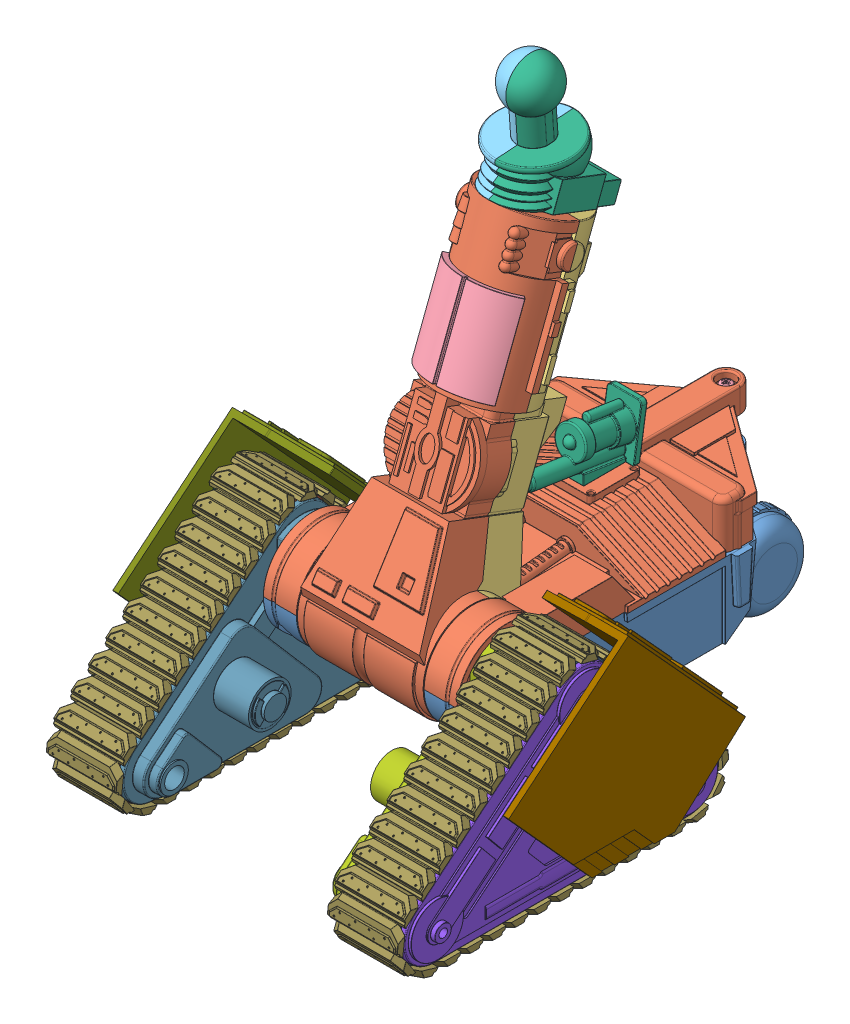
SolidWorks assembly Lower Portion, configuration Painted. Lengths in mm.
Overall size (141.8 212.73 199.77).
62 component instances, 24 part files, 21 mates.
Components (placement in the parent):
- Cradle Base-1: Cradle Base [Painted] at origin size (75.5 61.75 136.84)
  - Cradle Base (Lower)-1: Cradle Base (Lower) [Painted] at (0 27.3 0) size (75.5 28.26 136.84)
  - Cradle Base (Upper)-1: Cradle Base (Upper) [Default] at (0 27.3 0) size (71.63 21.58 136)
  - Cheese Head Thread-Forming Screw 2.8mm x 8mm-1: Cheese Head Thread-Forming Screw 2.8mm x 8mm [Default] at (-26 31.2 -19.6629) x (-1 0 0) z (0 0 1) size (5.45 9.97 5.45)
  - Cheese Head Thread-Forming Screw 2.8mm x 8mm-2: Cheese Head Thread-Forming Screw 2.8mm x 8mm [Default] at (26 31.2 -19.6629) x (-1 0 0) z (0 0 1) size (5.45 9.97 5.45)
  - Cheese Head Thread-Forming Screw 2.8mm x 8mm-3: Cheese Head Thread-Forming Screw 2.8mm x 8mm [Default] at (-26 31.2 -71.6629) x (-1 0 0) z (0 0 1) size (5.45 9.97 5.45)
  - Cheese Head Thread-Forming Screw 2.8mm x 8mm-4: Cheese Head Thread-Forming Screw 2.8mm x 8mm [Default] at (26 31.2 -71.6629) x (-1 0 0) z (0 0 1) size (5.45 9.97 5.45)
  - Cheese Head Thread-Forming Screw 2.5mm x 7mm-1: Cheese Head Thread-Forming Screw 2.5mm x 7mm [Default] at (-30.15 30.9 12.9371) x (-1 0 0) z (0 0 1) size (4.31 9.04 4.31)
  - Cheese Head Thread-Forming Screw 2.5mm x 7mm-2: Cheese Head Thread-Forming Screw 2.5mm x 7mm [Default] at (30.15 30.9 12.9371) x (-1 0 0) z (0 0 1) size (4.31 9.04 4.31)
  - Battery Door-1: Battery Door [Default] at (0 -0.48 -41.1629) size (62.19 4.7 51.07)
  - Cheese Head Thread-Forming Screw 2.5mm x 7mm-3: Cheese Head Thread-Forming Screw 2.5mm x 7mm [Default] at (0 9.07 -66.7129) x (-1 0 0) z (0 0 1) size (4.31 9.04 4.31)
  - Lower Torso Actuator-1: Lower Torso Actuator [Default] at (0 42.03 -59.2208) size (12.4 26.14 46.85)
- TDRV (Left)-1: TDRV (Left) [Default] at (50.325 -9.1697 53.1758) size (51.05 82.74 123.21)
  - Track Drive Side (Left, Inner)-1: Track Drive Side (Left, Inner) [Default] at (-11.975 -11 -45.5) size (22.2 65.97 113)
  - Track Drive Side (Left, Outer)-1: Track Drive Side (Left, Outer) [Default] at (11.975 -11 -45.5) size (26.75 65.97 113)
  - TDRV Beauty Cover (Left)-1: TDRV Beauty Cover (Left) [Default] at (20.575 -4.6199 -48.4187) x (1 0 0) z (0 -0.001763 0.999998) size (32.9 69.17 84.78)
  - Roller-1: Roller [Default] x (1 0 0) z (0 -0.637242 0.770664) size (18.92 25.7 25.7)
    - Roller (Female)-1: Roller (Female) [Default] at (5.16 0 0) size (10.22 25.7 25.7)
    - Roller (Male)-1: Roller (Male) [Default] at (-5.16 0 0) size (13 25.7 25.7)
  - Roller-2: Roller [Default] at (0 0 -91) x (1 0 0) z (0 1 0) size (18.92 25.7 25.7)
    - Roller (Female)-1: Roller (Female) [Default] at (5.16 0 0) size (10.22 25.7 25.7)
    - Roller (Male)-1: Roller (Male) [Default] at (-5.16 0 0) size (13 25.7 25.7)
  - Roller-3: Roller [Default] at (0 43.9697 -53.1758) x (1 0 0) z (0 -0.637242 0.770664) size (18.92 25.7 25.7)
    - Roller (Female)-1: Roller (Female) [Default] at (5.16 0 0) size (10.22 25.7 25.7)
    - Roller (Male)-1: Roller (Male) [Default] at (-5.16 0 0) size (13 25.7 25.7)
  - Treads-1: Treads [Default] at (0 -11 -45.5) size (25 72.41 119.4)
  - Cheese Head Thread-Forming Screw 2.8mm x 8mm-1: Cheese Head Thread-Forming Screw 2.8mm x 8mm [Default] at (-4.275 0 0) x (0 1 0) z (0 0 1) size (5.45 9.97 5.45)
  - Cheese Head Thread-Forming Screw 2.8mm x 8mm-3: Cheese Head Thread-Forming Screw 2.8mm x 8mm [Default] at (-4.275 0 -91) x (0 1 0) z (0 0 1) size (5.45 9.97 5.45)
  - Cheese Head Thread-Forming Screw 2.8mm x 8mm-7: Cheese Head Thread-Forming Screw 2.8mm x 8mm [Default] at (-4.275 43.9697 -53.1758) x (0 -1 0) z (0 0 -1) size (5.45 9.97 5.45)
  - Washer Head Thread-Forming Screw 2.6mm x 6mm-1: Washer Head Thread-Forming Screw 2.6mm x 6mm [Default] at (-18.575 36.4697 -53.1758) x (0 1 0) z (0 0 1) size (7.8 7.44 7.8)
- TDRV (Right)-1: TDRV (Right) [Default] at (-50.325 -9.1697 53.1758) size (51.05 82.74 123.21)
  - Track Drive Side (Right, Inner)-1: Track Drive Side (Right, Inner) [Default] at (11.975 -11 -45.5) size (22.2 65.97 113)
  - Track Drive Side (Right, Outer)-1: Track Drive Side (Right, Outer) [Default] at (-11.975 -11 -45.5) size (26.75 65.97 113)
  - TDRV Beauty Cover (Right)-1: TDRV Beauty Cover (Right) [Default] at (-20.575 -4.6199 -48.4187) x (1 0 0) z (0 -0.001763 0.999998) size (32.9 69.17 84.78)
  - Roller-1: Roller [Default] x (-1 0 0) z (0 0.637242 -0.770664) size (18.92 25.7 25.7)
    - Roller (Female)-1: Roller (Female) [Default] at (5.16 0 0) size (10.22 25.7 25.7)
    - Roller (Male)-1: Roller (Male) [Default] at (-5.16 0 0) size (13 25.7 25.7)
  - Roller-3: Roller [Default] at (0 0 -91) x (-1 0 0) z (0 -1 0) size (18.92 25.7 25.7)
    - Roller (Female)-1: Roller (Female) [Default] at (5.16 0 0) size (10.22 25.7 25.7)
    - Roller (Male)-1: Roller (Male) [Default] at (-5.16 0 0) size (13 25.7 25.7)
  - Roller-2: Roller [Default] at (0 43.9697 -53.1758) x (-1 0 0) z (0 -0.637242 0.770664) size (18.92 25.7 25.7)
    - Roller (Female)-1: Roller (Female) [Default] at (5.16 0 0) size (10.22 25.7 25.7)
    - Roller (Male)-1: Roller (Male) [Default] at (-5.16 0 0) size (13 25.7 25.7)
  - Treads-1: Treads [Default] at (0 -11 -45.5) size (25 72.41 119.4)
  - Washer Head Thread-Forming Screw 2.6mm x 6mm-1: Washer Head Thread-Forming Screw 2.6mm x 6mm [Default] at (18.575 36.4697 -53.1758) x (0 -1 0) z (0 0 1) size (7.8 7.44 7.8)
  - Cheese Head Thread-Forming Screw 2.8mm x 8mm-1: Cheese Head Thread-Forming Screw 2.8mm x 8mm [Default] at (4.275 0 0) x (0 -1 0) z (0 0 1) size (5.45 9.97 5.45)
  - Cheese Head Thread-Forming Screw 2.8mm x 8mm-5: Cheese Head Thread-Forming Screw 2.8mm x 8mm [Default] at (4.275 0 -91) x (0 -1 0) z (0 0 1) size (5.45 9.97 5.45)
  - Cheese Head Thread-Forming Screw 2.8mm x 8mm-6: Cheese Head Thread-Forming Screw 2.8mm x 8mm [Default] at (4.275 43.9697 -53.1758) x (0 -1 0) z (0 0 1) size (5.45 9.97 5.45)
- Caster-1: Caster [Default] at (0 -5.1622 -113.5) size (34.04 62.27 30)
  - Spindle-1: Spindle [Default] at origin size (10.68 53 11.45)
  - Caster (Female)-1: Caster (Female) [Default] at (-9.82 0 0) size (22.75 30 30)
  - Caster (Male)-1: Caster (Male) [Default] at (9.82 0 0) size (17.75 30 30)
- Lower Torso-1: Lower Torso [Default] at (0 27.3 0) x (1 0 0) z (0 0.358368 0.93358) size (51 138.12 43.66)
  - Lower Torso (Front)-1: Lower Torso (Front) [Default] at origin size (51 138.09 23.96)
  - Lower Torso (Rear)-1: Lower Torso (Rear) [Default] at origin size (51 138.12 23.19)
  - Console Door-1: Console Door [Default] at (0 83.2913 -1.8875) size (29.64 30.02 11.11)
  - Cheese Head Thread-Forming Screw 2.8mm x 8mm-1: Cheese Head Thread-Forming Screw 2.8mm x 8mm [Default] at (0 108.1913 2.0222) x (1 0 0) z (0 1 0) size (5.45 9.97 5.45)
  - Cheese Head Thread-Forming Screw 2.8mm x 8mm-2: Cheese Head Thread-Forming Screw 2.8mm x 8mm [Default] at (0 27.8913 2.0222) x (1 0 0) z (0 1 0) size (5.45 9.97 5.45)
- Waist-1: Waist [Default] at (0 133.7905 -42.8997) x (1 0 0) z (0 0.358368 0.93358) size (28.5 46.65 41.88)
  - Waist (Right)-1: Waist (Right) [Default] at origin size (18.75 46.65 41.88)
  - Waist (Left)-1: Waist (Left) [Default] at origin size (16.85 46.65 41.88)
- Cheese Head Thread-Forming Screw 2.5mm x 7mm-1: Cheese Head Thread-Forming Screw 2.5mm x 7mm [Default] at (0 36.83 -113.5) size (4.31 9.04 4.31)
Mates (geometry in assembly coordinates):
- CASTER ROTATION LOCK: parallel aligned: plane of Caster-1/Spindle-1 through (0 -5.1622 -113.5) normal (1 0 0); plane of assembly through (0 0 0) normal (1 0 0)
- TDRV ROTATION LOCK: parallel aligned: plane of TDRV (Left)-1 through (50.325 -9.1697 53.1758) normal (0 1 0); plane of assembly through (0 0 0) normal (0 1 0)
- Coincident1: coincident: plane of Cradle Base-1 through (0 0 0) normal (1 0 0); plane of assembly through (0 0 0) normal (1 0 0)
- Coincident2: coincident: plane of Cradle Base-1 through (0 0 0) normal (0 1 0); plane of assembly through (0 0 0) normal (0 1 0)
- Coincident3: coincident aligned: plane of Cradle Base-1 through (0 0 0) normal (0 0 1); plane of assembly through (0 0 0) normal (0 0 1)
- Concentric1: concentric aligned: cylinder of ? through (28.95 27.3 0) axis (1 0 0) radius 15.55; cylinder of TDRV (Left)-1/Track Drive Side (Left, Inner)-1 through (-20.6441 27.3 0) axis (1 0 0) radius 15
- Coincident4: coincident anti-aligned: plane of ? through (25.95 27.3 0) normal (-1 0 0); plane of TDRV (Left)-1/Washer Head Thread-Forming Screw 2.6mm x 6mm-1 through (25.95 26 0) normal (1 0 0)
- Concentric2: concentric anti-aligned: cylinder of ? through (0 0 -113.5) axis (0 1 0) radius 3; cylinder of Caster-1/Spindle-1 through (0 42.1128 -113.5) axis (0 -1 0) radius 2.675
- Coincident6: coincident anti-aligned: plane of ? through (0 42.1128 0) normal (0 -1 0); plane of Caster-1/Spindle-1 through (0 42.1128 -113.5) normal (0 1 0)
- Concentric4: concentric aligned: cylinder of ? through (-28.95 27.3 0) axis (-1 0 0) radius 15.55; cylinder of TDRV (Right)-1/Track Drive Side (Right, Inner)-1 through (20.6441 27.3 0) axis (-1 0 0) radius 15
- Coincident7: coincident aligned: plane of TDRV (Left)-1 through (50.325 -9.1697 53.1758) normal (0 1 0); plane of TDRV (Right)-1 through (-50.325 -9.1697 53.1758) normal (0 1 0)
- Coincident9: coincident anti-aligned: plane of ? through (-25.95 27.3 0) normal (1 0 0); plane of TDRV (Right)-1/Washer Head Thread-Forming Screw 2.6mm x 6mm-1 through (-25.95 28.6 0) normal (-1 0 0)
- Concentric5: concentric aligned: cylinder of Caster-1/Spindle-1 through (0 42.1128 -113.5) axis (0 1 0) radius 1.025; cylinder of Cheese Head Thread-Forming Screw 2.5mm x 7mm-1 through (0 45.83 -113.5) axis (0 1 0) radius 1.25
- Coincident10: coincident anti-aligned: plane of ? through (0 44.23 -113.5) normal (0 1 0); plane of Cheese Head Thread-Forming Screw 2.5mm x 7mm-1 through (-1.25 44.23 -113.5) normal (0 -1 0)
- Coincident11: coincident aligned: plane of Caster-1/Spindle-1 through (0 -5.1622 -113.5) normal (1 0 0); plane of Cheese Head Thread-Forming Screw 2.5mm x 7mm-1 through (0 36.83 -113.5) normal (1 0 0)
- Concentric6: concentric anti-aligned: cylinder of ? through (0 133.7905 -42.8997) axis (0 0.93358 -0.358368) radius 8; cylinder of ? through (0 138.4584 -44.6915) axis (0 -0.93358 0.358368) radius 7.9
- Coincident12: coincident anti-aligned: plane of ? through (0 138.4584 -44.6915) normal (0 0.93358 -0.358368); plane of ? through (0 138.4584 -44.6915) normal (0 -0.93358 0.358368)
- Coincident13: coincident aligned: plane of ?; plane of ?
- Concentric7: concentric aligned: cylinder of ? through (24.2019 27.3 0) axis (-1 0 0) radius 16.6; cylinder of ? through (70.482 27.3 0) axis (-1 0 0) radius 15.55
- Coincident14: coincident aligned: plane of Cradle Base-1 through (0 0 0) normal (1 0 0); plane of ?
- Angle1: planar angle = 1.204277 rad aligned: plane of ? through (0 27.3 0) normal (0 0.358368 0.93358); plane of assembly through (0 0 0) normal (0 1 0)
